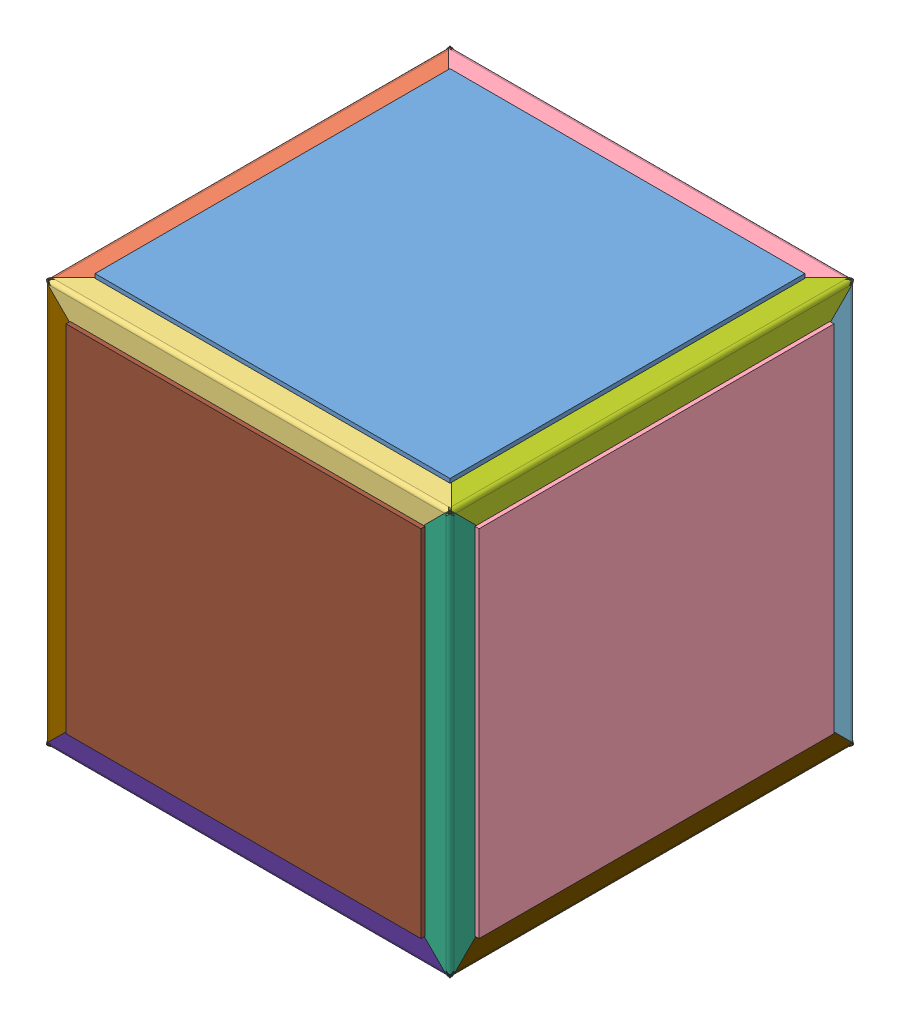
SolidWorks assembly cube_02, configuration cube02. Lengths in mm.
Overall size (158.12 158.12 158.12).
30 component instances, 30 part files, 92 mates.
Components (placement in the parent):
- pr^cube_02-28: pr^cube_02 [cube01] x (-1 0 0) z (0 0 1) size (135.89 1.59 135.89) (virtual)
- dr1^cube_02-55: dr1^cube_02 [cube01] at (-76.8646 77.47 0) x (0 -1 0) z (0 0 1) size (26.01 26.01 154.95) (virtual)
- dr2^cube_02-37: dr2^cube_02 [cube01] at (0 77.47 76.8646) x (0 -1 0) z (1 0 0) size (26.01 26.01 154.95) (virtual)
- dr3^cube_02-33: dr3^cube_02 [cube01] at (0 77.47 -76.8646) x (0 -1 0) z (-1 0 0) size (26.01 26.01 154.95) (virtual)
- br1^cube_02-49: br1^cube_02 [Default] at (0 52.07 -52.07) x (0 0 1) z (-1 0 0) size (50.8 50.8 97.03) (virtual)
- br2^cube_02-61: br2^cube_02 [Default] at (-52.07 52.07 0) size (50.8 50.8 97.03) (virtual)
- br3^cube_02-46: br3^cube_02 [Default] at (0 52.07 52.07) x (0 0 -1) z (1 0 0) size (50.8 50.8 97.03) (virtual)
- pg^cube_02-20: pg^cube_02 [cube01] x (0 -1 0) z (0 0 1) size (135.89 1.59 135.89) (virtual)
- dg1^cube_02-38: dg1^cube_02 [cube01] at (-77.47 0 76.8646) x (1 0 0) z (0 1 0) size (26.01 26.01 154.95) (virtual)
- dg2^cube_02-41: dg2^cube_02 [cube01] at (-77.47 -76.8646 0) size (26.01 26.01 154.95) (virtual)
- dg3^cube_02-34: dg3^cube_02 [cube01] at (-77.47 0 -76.8646) x (1 0 0) z (0 -1 0) size (26.01 26.01 154.95) (virtual)
- bg1^cube_02-47: bg1^cube_02 [Default] at (-52.07 -52.07 0) x (0 1 0) z (0 0 1) size (50.8 50.8 97.03) (virtual)
- bg2^cube_02-44: bg2^cube_02 [Default] at (-52.07 0 52.07) x (0 0 -1) z (0 1 0) size (50.8 50.8 97.03) (virtual)
- bg3^cube_02-40: bg3^cube_02 [Default] at (-52.07 0 -52.07) x (0 0 1) z (0 -1 0) size (50.8 50.8 97.03) (virtual)
- py^cube_02-21: py^cube_02 [cube01] at origin size (135.89 1.59 135.89) (virtual)
- dy1^cube_02-35: dy1^cube_02 [cube01] at (0 -77.47 -76.8646) x (0 1 0) z (1 0 0) size (26.01 26.01 154.95) (virtual)
- dy2^cube_02-39: dy2^cube_02 [cube01] at (0 -77.47 76.8646) x (0 1 0) z (-1 0 0) size (26.01 26.01 154.95) (virtual)
- dy3^cube_02-42: dy3^cube_02 [cube01] at (76.8646 -77.47 0) x (0 1 0) z (0 0 1) size (26.01 26.01 154.95) (virtual)
- by1^cube_02-41: by1^cube_02 [Default] at (0 -52.07 -52.07) x (0 0 1) z (1 0 0) size (50.8 50.8 97.03) (virtual)
- by2^cube_02-45: by2^cube_02 [Default] at (0 -52.07 52.07) x (0 0 -1) z (-1 0 0) size (50.8 50.8 97.03) (virtual)
- by3^cube_02-48: by3^cube_02 [Default] at (52.07 -52.07 0) x (-1 0 0) z (0 0 1) size (50.8 50.8 97.03) (virtual)
- po^cube_02-22: po^cube_02 [cube01] x (0 1 0) z (0 0 1) size (135.89 1.59 135.89) (virtual)
- do1^cube_02-36: do1^cube_02 [cube01] at (77.47 0 -76.8646) x (-1 0 0) z (0 1 0) size (26.01 26.01 154.95) (virtual)
- do2^cube_02-40: do2^cube_02 [cube01] at (77.47 0 76.8646) x (-1 0 0) z (0 -1 0) size (26.01 26.01 154.95) (virtual)
- do3^cube_02-47: do3^cube_02 [cube01] at (77.47 76.8646 0) x (-1 0 0) z (0 0 1) size (26.01 26.01 154.95) (virtual)
- bo1^cube_02-42: bo1^cube_02 [Default] at (52.07 0 -52.07) x (0 0 1) z (0 1 0) size (50.8 50.8 97.03) (virtual)
- bo2^cube_02-46: bo2^cube_02 [Default] at (52.07 0 52.07) x (0 0 -1) z (0 -1 0) size (50.8 50.8 97.03) (virtual)
- bo3^cube_02-62: bo3^cube_02 [Default] at (52.07 52.07 0) x (0 -1 0) z (0 0 1) size (50.8 50.8 97.03) (virtual)
- pc^cube_02-18: pc^cube_02 [cube01] x (-1 0 0) z (0 -1 0) size (135.89 1.59 135.89) (virtual)
- pb^cube_02-21: pb^cube_02 [cube01] x (-1 0 0) z (0 1 0) size (135.89 1.59 135.89) (virtual)
Mates (geometry in assembly coordinates):
- Coincident1: coincident anti-aligned: plane of pr^cube_02-28 through (67.945 77.47 -67.945) normal (0 -1 0); plane of br1^cube_02-49 through (-48.514 77.47 -52.07) normal (0 1 0)
- Coincident2: coincident anti-aligned: plane of pr^cube_02-28 through (67.945 77.47 -67.945) normal (0 -1 0); plane of br2^cube_02-61 through (-52.07 77.47 48.514) normal (0 1 0)
- Coincident3: coincident anti-aligned: plane of pr^cube_02-28 through (67.945 77.47 -67.945) normal (0 -1 0); plane of br3^cube_02-46 through (48.514 77.47 52.07) normal (0 1 0)
- Coincident4: coincident anti-aligned: plane of pr^cube_02-28 through (67.945 77.47 -67.945) normal (0 -1 0); plane of bo3^cube_02-62 through (52.07 77.47 48.514) normal (0 1 0)
- Coincident5: coincident anti-aligned: plane of pr^cube_02-28 through (67.945 77.47 -67.945) normal (0 -1 0); plane of dr3^cube_02-33 through (0 77.47 -154.3346) normal (0 1 0)
- Coincident6: coincident anti-aligned: plane of pr^cube_02-28 through (67.945 77.47 -67.945) normal (0 -1 0); plane of dr1^cube_02-55 through (-154.3346 77.47 0) normal (0 1 0)
- Coincident7: coincident anti-aligned: plane of pr^cube_02-28 through (67.945 77.47 -67.945) normal (0 -1 0); plane of do3^cube_02-47 through (-0.6054 77.47 0) normal (0 1 0)
- Coincident8: coincident anti-aligned: plane of pr^cube_02-28 through (67.945 77.47 -67.945) normal (0 -1 0); plane of dr2^cube_02-37 through (0 77.47 154.3346) normal (0 1 0)
- Coincident34: coincident anti-aligned: plane of pb^cube_02-21 through (67.945 -67.945 -77.47) normal (0 0 1); plane of by1^cube_02-41 through (48.514 -52.07 -77.47) normal (0 0 -1)
- Coincident35: coincident anti-aligned: plane of pb^cube_02-21 through (67.945 -67.945 -77.47) normal (0 0 1); plane of bo1^cube_02-42 through (52.07 48.514 -77.47) normal (0 0 -1)
- Coincident36: coincident anti-aligned: plane of pb^cube_02-21 through (67.945 -67.945 -77.47) normal (0 0 1); plane of br1^cube_02-49 through (-48.514 52.07 -77.47) normal (0 0 -1)
- Coincident37: coincident anti-aligned: plane of pb^cube_02-21 through (67.945 -67.945 -77.47) normal (0 0 1); plane of bg3^cube_02-40 through (-52.07 -48.514 -77.47) normal (0 0 -1)
- Coincident38: coincident anti-aligned: plane of pb^cube_02-21 through (67.945 -67.945 -77.47) normal (0 0 1); plane of dg3^cube_02-34 through (0.6054 0 -77.47) normal (0 0 -1)
- Coincident39: coincident anti-aligned: plane of pb^cube_02-21 through (67.945 -67.945 -77.47) normal (0 0 1); plane of dr3^cube_02-33 through (0 -0.6054 -77.47) normal (0 0 -1)
- Coincident40: coincident anti-aligned: plane of pb^cube_02-21 through (67.945 -67.945 -77.47) normal (0 0 1); plane of do1^cube_02-36 through (-0.6054 0 -77.47) normal (0 0 -1)
- Coincident41: coincident anti-aligned: plane of pb^cube_02-21 through (67.945 -67.945 -77.47) normal (0 0 1); plane of dy1^cube_02-35 through (0 0.6054 -77.47) normal (0 0 -1)
- Coincident42: coincident anti-aligned: plane of pc^cube_02-18 through (67.945 67.945 77.47) normal (0 0 -1); plane of bo2^cube_02-46 through (52.07 -48.514 77.47) normal (0 0 1)
- Coincident43: coincident anti-aligned: plane of pc^cube_02-18 through (67.945 67.945 77.47) normal (0 0 -1); plane of br3^cube_02-46 through (48.514 52.07 77.47) normal (0 0 1)
- Coincident44: coincident anti-aligned: plane of pc^cube_02-18 through (67.945 67.945 77.47) normal (0 0 -1); plane of bg2^cube_02-44 through (-52.07 48.514 77.47) normal (0 0 1)
- Coincident45: coincident anti-aligned: plane of pc^cube_02-18 through (67.945 67.945 77.47) normal (0 0 -1); plane of by2^cube_02-45 through (-48.514 -52.07 77.47) normal (0 0 1)
- Coincident46: coincident anti-aligned: plane of pc^cube_02-18 through (67.945 67.945 77.47) normal (0 0 -1); plane of do2^cube_02-40 through (-0.6054 0 77.47) normal (0 0 1)
- Coincident47: coincident anti-aligned: plane of pc^cube_02-18 through (67.945 67.945 77.47) normal (0 0 -1); plane of dy2^cube_02-39 through (0 0.6054 77.47) normal (0 0 1)
- Coincident48: coincident anti-aligned: plane of pc^cube_02-18 through (67.945 67.945 77.47) normal (0 0 -1); plane of dg1^cube_02-38 through (0.6054 0 77.47) normal (0 0 1)
- Coincident49: coincident anti-aligned: plane of pc^cube_02-18 through (67.945 67.945 77.47) normal (0 0 -1); plane of dr2^cube_02-37 through (0 -0.6054 77.47) normal (0 0 1)
- Coincident50: coincident anti-aligned: plane of pg^cube_02-20 through (-77.47 67.945 -67.945) normal (1 0 0); plane of bg3^cube_02-40 through (-77.47 -48.514 -52.07) normal (-1 0 0)
- Coincident51: coincident anti-aligned: plane of pg^cube_02-20 through (-77.47 67.945 -67.945) normal (1 0 0); plane of bg1^cube_02-47 through (-77.47 -52.07 48.514) normal (-1 0 0)
- Coincident52: coincident anti-aligned: plane of pg^cube_02-20 through (-77.47 67.945 -67.945) normal (1 0 0); plane of bg2^cube_02-44 through (-77.47 48.514 52.07) normal (-1 0 0)
- Coincident53: coincident anti-aligned: plane of pg^cube_02-20 through (-77.47 67.945 -67.945) normal (1 0 0); plane of dr1^cube_02-55 through (-77.47 -0.6054 0) normal (-1 0 0)
- Coincident54: coincident anti-aligned: plane of pg^cube_02-20 through (-77.47 67.945 -67.945) normal (1 0 0); plane of dg3^cube_02-34 through (-77.47 0 -154.3346) normal (-1 0 0)
- Coincident55: coincident anti-aligned: plane of pg^cube_02-20 through (-77.47 67.945 -67.945) normal (1 0 0); plane of dg2^cube_02-41 through (-77.47 -154.3346 0) normal (-1 0 0)
- Coincident56: coincident anti-aligned: plane of pg^cube_02-20 through (-77.47 67.945 -67.945) normal (1 0 0); plane of dg1^cube_02-38 through (-77.47 0 154.3346) normal (-1 0 0)
- Coincident99: coincident anti-aligned: plane of pg^cube_02-20 through (-77.47 67.945 -67.945) normal (1 0 0); plane of br2^cube_02-61 through (-77.47 52.07 48.514) normal (-1 0 0)
- Coincident57: coincident anti-aligned: plane of py^cube_02-21 through (-67.945 -77.47 -67.945) normal (0 1 0); plane of by3^cube_02-48 through (52.07 -77.47 48.514) normal (0 -1 0)
- Coincident58: coincident anti-aligned: plane of py^cube_02-21 through (-67.945 -77.47 -67.945) normal (0 1 0); plane of by2^cube_02-45 through (-48.514 -77.47 52.07) normal (0 -1 0)
- Coincident59: coincident anti-aligned: plane of py^cube_02-21 through (-67.945 -77.47 -67.945) normal (0 1 0); plane of bg1^cube_02-47 through (-52.07 -77.47 48.514) normal (0 -1 0)
- Coincident60: coincident anti-aligned: plane of py^cube_02-21 through (-67.945 -77.47 -67.945) normal (0 1 0); plane of by1^cube_02-41 through (48.514 -77.47 -52.07) normal (0 -1 0)
- Coincident61: coincident anti-aligned: plane of py^cube_02-21 through (-67.945 -77.47 -67.945) normal (0 1 0); plane of dy3^cube_02-42 through (154.3346 -77.47 0) normal (0 -1 0)
- Coincident62: coincident anti-aligned: plane of py^cube_02-21 through (-67.945 -77.47 -67.945) normal (0 1 0); plane of dy2^cube_02-39 through (0 -77.47 154.3346) normal (0 -1 0)
- Coincident63: coincident anti-aligned: plane of py^cube_02-21 through (-67.945 -77.47 -67.945) normal (0 1 0); plane of dg2^cube_02-41 through (0.6054 -77.47 0) normal (0 -1 0)
- Coincident64: coincident anti-aligned: plane of py^cube_02-21 through (-67.945 -77.47 -67.945) normal (0 1 0); plane of dy1^cube_02-35 through (0 -77.47 -154.3346) normal (0 -1 0)
- Coincident65: coincident anti-aligned: plane of po^cube_02-22 through (77.47 -67.945 -67.945) normal (-1 0 0); plane of bo1^cube_02-42 through (77.47 48.514 -52.07) normal (1 0 0)
- Coincident66: coincident anti-aligned: plane of po^cube_02-22 through (77.47 -67.945 -67.945) normal (-1 0 0); plane of by3^cube_02-48 through (77.47 -52.07 48.514) normal (1 0 0)
- Coincident67: coincident anti-aligned: plane of po^cube_02-22 through (77.47 -67.945 -67.945) normal (-1 0 0); plane of bo2^cube_02-46 through (77.47 -48.514 52.07) normal (1 0 0)
- Coincident68: coincident anti-aligned: plane of po^cube_02-22 through (77.47 -67.945 -67.945) normal (-1 0 0); plane of bo3^cube_02-62 through (77.47 52.07 48.514) normal (1 0 0)
- Coincident69: coincident anti-aligned: plane of po^cube_02-22 through (77.47 -67.945 -67.945) normal (-1 0 0); plane of do2^cube_02-40 through (77.47 0 154.3346) normal (1 0 0)
- Coincident70: coincident anti-aligned: plane of po^cube_02-22 through (77.47 -67.945 -67.945) normal (-1 0 0); plane of do3^cube_02-47 through (77.47 154.3346 0) normal (1 0 0)
- Coincident71: coincident anti-aligned: plane of po^cube_02-22 through (77.47 -67.945 -67.945) normal (-1 0 0); plane of do1^cube_02-36 through (77.47 0 -154.3346) normal (1 0 0)
- Coincident72: coincident anti-aligned: plane of po^cube_02-22 through (77.47 -67.945 -67.945) normal (-1 0 0); plane of dy3^cube_02-42 through (77.47 0.6054 0) normal (1 0 0)
- Coincident73: coincident aligned: plane of assembly through (0 0 0) normal (0 0 1); plane of dy3^cube_02-42 through (76.8646 -77.47 0) normal (0 0 1)
- Coincident74: coincident aligned: plane of assembly through (0 0 0) normal (0 0 1); plane of by3^cube_02-48 through (52.07 -52.07 0) normal (0 0 1)
- Coincident75: coincident aligned: plane of assembly through (0 0 0) normal (0 0 1); plane of bo3^cube_02-62 through (52.07 52.07 0) normal (0 0 1)
- Coincident76: coincident aligned: plane of assembly through (0 0 0) normal (0 0 1); plane of do3^cube_02-47 through (77.47 76.8646 0) normal (0 0 1)
- Coincident77: coincident aligned: plane of assembly through (0 0 0) normal (0 0 1); plane of dg2^cube_02-41 through (-77.47 -76.8646 0) normal (0 0 1)
- Coincident78: coincident aligned: plane of assembly through (0 0 0) normal (0 0 1); plane of bg1^cube_02-47 through (-52.07 -52.07 0) normal (0 0 1)
- Coincident79: coincident aligned: plane of assembly through (0 0 0) normal (0 0 1); plane of dr1^cube_02-55 through (-76.8646 77.47 0) normal (0 0 1)
- Coincident80: coincident aligned: plane of assembly through (0 0 0) normal (0 0 1); plane of br2^cube_02-61 through (-52.07 52.07 0) normal (0 0 1)
- Coincident81: coincident aligned: plane of assembly through (0 0 0) normal (0 1 0); plane of bo1^cube_02-42 through (52.07 0 -52.07) normal (0 1 0)
- Coincident82: coincident aligned: plane of assembly through (0 0 0) normal (0 1 0); plane of py^cube_02-21 through (0 0 0) normal (0 1 0)
- Coincident83: coincident aligned: plane of assembly through (0 0 0) normal (0 1 0); plane of do1^cube_02-36 through (77.47 0 -76.8646) normal (0 1 0)
- Coincident84: coincident anti-aligned: plane of assembly through (0 0 0) normal (0 1 0); plane of bg3^cube_02-40 through (-52.07 0 -52.07) normal (0 -1 0)
- Coincident85: coincident anti-aligned: plane of assembly through (0 0 0) normal (0 1 0); plane of dg3^cube_02-34 through (-77.47 0 -76.8646) normal (0 -1 0)
- Coincident86: coincident aligned: plane of assembly through (0 0 0) normal (0 1 0); plane of dg1^cube_02-38 through (-77.47 0 76.8646) normal (0 1 0)
- Coincident87: coincident aligned: plane of assembly through (0 0 0) normal (0 1 0); plane of bg2^cube_02-44 through (-52.07 0 52.07) normal (0 1 0)
- Coincident88: coincident anti-aligned: plane of assembly through (0 0 0) normal (0 1 0); plane of bo2^cube_02-46 through (52.07 0 52.07) normal (0 -1 0)
- Coincident89: coincident anti-aligned: plane of assembly through (0 0 0) normal (0 1 0); plane of do2^cube_02-40 through (77.47 0 76.8646) normal (0 -1 0)
- Coincident90: coincident anti-aligned: plane of assembly through (0 0 0) normal (1 0 0); plane of by2^cube_02-45 through (0 -52.07 52.07) normal (-1 0 0)
- Coincident91: coincident anti-aligned: plane of assembly through (0 0 0) normal (1 0 0); plane of dy2^cube_02-39 through (0 -77.47 76.8646) normal (-1 0 0)
- Coincident92: coincident aligned: plane of assembly through (0 0 0) normal (1 0 0); plane of pg^cube_02-20
- Coincident93: coincident aligned: plane of assembly through (0 0 0) normal (1 0 0); plane of dr2^cube_02-37 through (0 77.47 76.8646) normal (1 0 0)
- Coincident94: coincident aligned: plane of assembly through (0 0 0) normal (1 0 0); plane of br3^cube_02-46 through (0 52.07 52.07) normal (1 0 0)
- Coincident95: coincident anti-aligned: plane of assembly through (0 0 0) normal (1 0 0); plane of dr3^cube_02-33 through (0 77.47 -76.8646) normal (-1 0 0)
- Coincident96: coincident anti-aligned: plane of assembly through (0 0 0) normal (1 0 0); plane of br1^cube_02-49 through (0 52.07 -52.07) normal (-1 0 0)
- Coincident97: coincident aligned: plane of assembly through (0 0 0) normal (1 0 0); plane of by1^cube_02-41 through (0 -52.07 -52.07) normal (1 0 0)
- Coincident98: coincident aligned: plane of assembly through (0 0 0) normal (1 0 0); plane of dy1^cube_02-35 through (0 -77.47 -76.8646) normal (1 0 0)
- Coincident100: coincident anti-aligned: plane of pr^cube_02-28; plane of assembly through (0 0 0) normal (1 0 0)
- Coincident101: coincident aligned: plane of pr^cube_02-28 through (0 0 0) normal (0 0 1); plane of assembly through (0 0 0) normal (0 0 1)
- Coincident102: coincident anti-aligned: plane of pr^cube_02-28; plane of assembly through (0 0 0) normal (0 1 0)
- Coincident106: coincident anti-aligned: plane of pg^cube_02-20; plane of assembly through (0 0 0) normal (0 1 0)
- Coincident107: coincident aligned: plane of pg^cube_02-20; plane of assembly through (0 0 0) normal (1 0 0)
- Coincident108: coincident aligned: plane of pg^cube_02-20 through (0 0 0) normal (0 0 1); plane of assembly through (0 0 0) normal (0 0 1)
- Coincident109: coincident aligned: plane of py^cube_02-21 through (0 0 0) normal (0 0 1); plane of assembly through (0 0 0) normal (0 0 1)
- Coincident110: coincident aligned: plane of py^cube_02-21 through (0 0 0) normal (0 1 0); plane of assembly through (0 0 0) normal (0 1 0)
- Coincident111: coincident aligned: plane of py^cube_02-21 through (0 0 0) normal (1 0 0); plane of assembly through (0 0 0) normal (1 0 0)
- Coincident112: coincident aligned: plane of po^cube_02-22 through (0 0 0) normal (0 0 1); plane of assembly through (0 0 0) normal (0 0 1)
- Coincident113: coincident anti-aligned: plane of po^cube_02-22; plane of assembly through (0 0 0) normal (1 0 0)
- Coincident114: coincident aligned: plane of po^cube_02-22; plane of assembly through (0 0 0) normal (0 1 0)
- Coincident115: coincident anti-aligned: plane of pc^cube_02-18 through (0 0 0) normal (0 -1 0); plane of assembly through (0 0 0) normal (0 1 0)
- Coincident116: coincident anti-aligned: plane of pc^cube_02-18; plane of assembly through (0 0 0) normal (0 0 1)
- Coincident117: coincident anti-aligned: plane of pc^cube_02-18; plane of assembly through (0 0 0) normal (1 0 0)
- Coincident118: coincident aligned: plane of pb^cube_02-21 through (0 0 0) normal (0 1 0); plane of assembly through (0 0 0) normal (0 1 0)
- Coincident119: coincident aligned: plane of pb^cube_02-21; plane of assembly through (0 0 0) normal (0 0 1)
- Coincident120: coincident anti-aligned: line of pb^cube_02-21 through (0.8731 -0.8731 0) axis (0 0 -1); plane of assembly through (0 0 0) normal (1 0 0)
